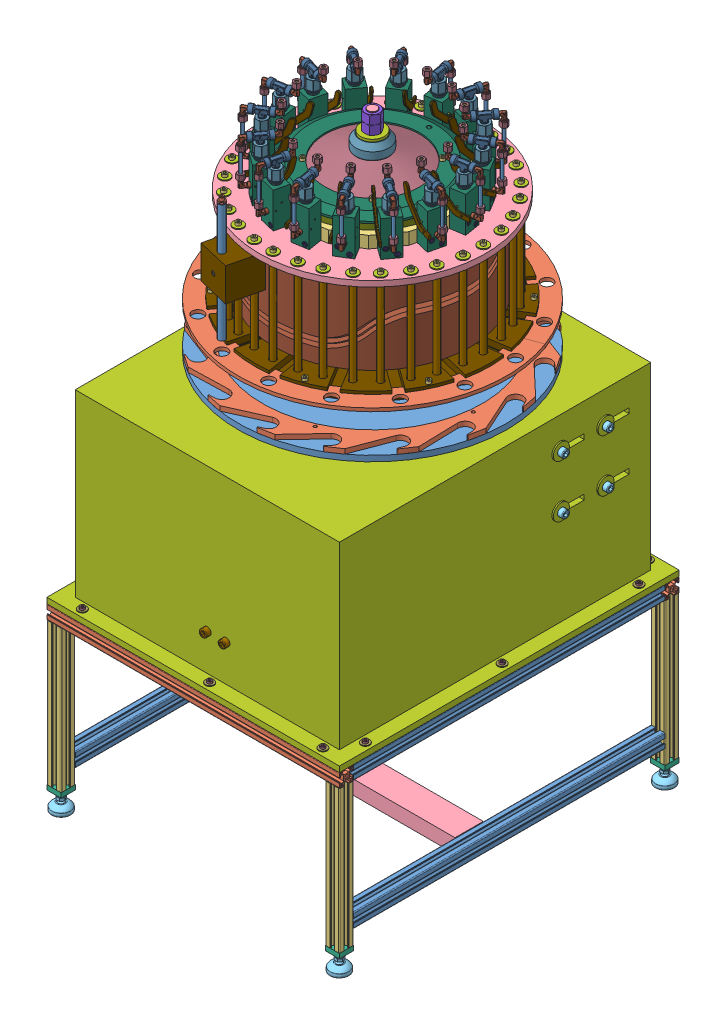
SolidWorks assembly Assieme_FINALE, configuration Default. Lengths in mm. (continued)
Components (placement in the parent): (continued)
- assieme parte rotante-2: assieme parte rotante [Default] at (-8.3038 623.9178 -528.0599) x (0 1 0) z (-0.913062 0 0.407822) size (749.63 778.63 778.63) (continued)
  - AssiemeValvola-15: AssiemeValvola [Default] at (515.3257 182.5711 371.0008) x (0 -0.965926 0.258819) z (0 0.258819 0.965926) size (90.26 138.63 38)
    - RaccordoT-1: RaccordoT [Default] at origin size (43 29.75 16.5)
    - Raccordo a L-1: Raccordo a L [Default] at (-30 0 0) x (0 -1 0) z (0 0 -1) size (28.34 25.51 14.01)
      - 1809_06_10_01-1: 1809_06_10_01 [Default] at origin size (22.49 23 10)
      - 1809_06_10_02-1: 1809_06_10_02 [Default] at origin size (6.5 8.5 8.5)
      - 1809_06_10_03-1: 1809_06_10_03 [Default] at origin size (11.02 15.01 14.01)
    - Raccordo a L-2: Raccordo a L [Default] at (30 0 0) x (0 1 0) z (0 0 -1) size (28.34 25.51 14.01)
      - 1809_06_10_01-1: 1809_06_10_01 [Default] at origin size (22.49 23 10)
      - 1809_06_10_02-1: 1809_06_10_02 [Default] at origin size (6.5 8.5 8.5)
      - 1809_06_10_03-1: 1809_06_10_03 [Default] at origin size (11.02 15.01 14.01)
    - TappoChiusura-1: TappoChiusura [Default] at (0 -32 0) x (0 -1 0) z (0 0 1) size (38.28 26.74 26.74)
    - CorpoValvola-1: CorpoValvola [Default] at (-15 -115.2824 0) size (30 75 34)
    - Raccordo a L-3: Raccordo a L [Default] at (-30 -88.2824 0) x (0 1 0) z (0 0 1) size (28.34 25.51 14.01)
      - 1809_06_10_01-1: 1809_06_10_01 [Default] at origin size (22.49 23 10)
      - 1809_06_10_02-1: 1809_06_10_02 [Default] at origin size (6.5 8.5 8.5)
      - 1809_06_10_03-1: 1809_06_10_03 [Default] at origin size (11.02 15.01 14.01)
    - Spina_3x38-1: Spina_3x38 [Default] at (0 -68.2824 -21) x (-1 0 0) z (0 0 1) size (3 3 38)
    - Spina_3x38-2: Spina_3x38 [Default] at (-10 -80.2824 -21) x (0.996193 0.087174 0) z (0 0 1) size (3 3 38)
    - M5 40mm-3: M5 40mm [ISO 4762 M5 x 40 - 40N] at (-14.6 -108.7824 9) size (45 8.5 8.5)
    - M5 40mm-2: M5 40mm [ISO 4762 M5 x 40 - 40N] at (-14.6 -96.7824 -9) size (45 8.5 8.5)
    - LevaValvola-1: LevaValvola [Default] at (-24.507 -86.571 -17) x (0.996193 0.087174 0) z (0 0 1) size (77.55 60.2 4)
    - Tubo-1: Tubo [Default] at (-30 -15.9665 0) x (1 0 0) z (0 -1 0) size (6 6 56.4)
  - AssiemeValvola-16: AssiemeValvola [Default] at (515.3257 153.2338 311.5106) x (0 -0.793353 0.608761) z (0 0.608761 0.793353) size (90.26 138.63 38)
    - RaccordoT-1: RaccordoT [Default] at origin size (43 29.75 16.5)
    - Raccordo a L-1: Raccordo a L [Default] at (-30 0 0) x (0 -1 0) z (0 0 -1) size (28.34 25.51 14.01)
      - 1809_06_10_01-1: 1809_06_10_01 [Default] at origin size (22.49 23 10)
      - 1809_06_10_02-1: 1809_06_10_02 [Default] at origin size (6.5 8.5 8.5)
      - 1809_06_10_03-1: 1809_06_10_03 [Default] at origin size (11.02 15.01 14.01)
    - Raccordo a L-2: Raccordo a L [Default] at (30 0 0) x (0 1 0) z (0 0 -1) size (28.34 25.51 14.01)
      - 1809_06_10_01-1: 1809_06_10_01 [Default] at origin size (22.49 23 10)
      - 1809_06_10_02-1: 1809_06_10_02 [Default] at origin size (6.5 8.5 8.5)
      - 1809_06_10_03-1: 1809_06_10_03 [Default] at origin size (11.02 15.01 14.01)
    - TappoChiusura-1: TappoChiusura [Default] at (0 -32 0) x (0 -1 0) z (0 0 1) size (38.28 26.74 26.74)
    - CorpoValvola-1: CorpoValvola [Default] at (-15 -115.2824 0) size (30 75 34)
    - Raccordo a L-3: Raccordo a L [Default] at (-30 -88.2824 0) x (0 1 0) z (0 0 1) size (28.34 25.51 14.01)
      - 1809_06_10_01-1: 1809_06_10_01 [Default] at origin size (22.49 23 10)
      - 1809_06_10_02-1: 1809_06_10_02 [Default] at origin size (6.5 8.5 8.5)
      - 1809_06_10_03-1: 1809_06_10_03 [Default] at origin size (11.02 15.01 14.01)
    - Spina_3x38-1: Spina_3x38 [Default] at (0 -68.2824 -21) x (-1 0 0) z (0 0 1) size (3 3 38)
    - Spina_3x38-2: Spina_3x38 [Default] at (-10 -80.2824 -21) x (0.996193 0.087174 0) z (0 0 1) size (3 3 38)
    - M5 40mm-3: M5 40mm [ISO 4762 M5 x 40 - 40N] at (-14.6 -108.7824 9) size (45 8.5 8.5)
    - M5 40mm-2: M5 40mm [ISO 4762 M5 x 40 - 40N] at (-14.6 -96.7824 -9) size (45 8.5 8.5)
    - LevaValvola-1: LevaValvola [Default] at (-24.507 -86.571 -17) x (0.996193 0.087174 0) z (0 0 1) size (77.55 60.2 4)
    - Tubo-1: Tubo [Default] at (-30 -15.9665 0) x (1 0 0) z (0 -1 0) size (6 6 56.4)
  - Disco alimentazione guarnizione fi24.4-1: Disco alimentazione guarnizione fi24.4 [Default] at (198.0433 18.3637 415) x (0 0.065403 0.997859) z (-1 0 0) size (570 285 7.35)
  - Disco alimentazione guarnizione fi24.4-2: Disco alimentazione guarnizione fi24.4 [Default] at (198.0433 18.3637 415) x (0 -0.065403 -0.997859) z (-1 0 0) size (570 285 7.35)
  - m6 12mm-1: m6 12mm [ISO 4762 M6 x 12 - 12N] at (210.0433 200.6849 574.8914) x (-1 0 0) z (0 0.793353 -0.608761) size (18 10 10)
  - m6 12mm-7: m6 12mm [ISO 4762 M6 x 12 - 12N] at (210.0433 260.3445 399.1397) x (-1 0 0) z (0 0.793353 -0.608761) size (18 10 10)
  - m6 12mm-8: m6 12mm [ISO 4762 M6 x 12 - 12N] at (210.0433 96.3128 185.3694) x (-1 0 0) z (0 0.793353 -0.608761) size (18 10 10)
  - m6 12mm-9: m6 12mm [ISO 4762 M6 x 12 - 12N] at (210.0433 -59.5854 644.6306) x (-1 0 0) z (0 -0.793353 -0.608761) size (18 10 10)
  - m6 12mm-10: m6 12mm [ISO 4762 M6 x 12 - 12N] at (210.0433 -223.6171 430.8603) x (-1 0 0) z (0 -0.793353 -0.608761) size (18 10 10)
  - m6 12mm-11: m6 12mm [ISO 4762 M6 x 12 - 12N] at (210.0433 -163.9575 255.1086) x (-1 0 0) z (0 0.793353 -0.608761) size (18 10 10)
- assieme parte fissa-1: assieme parte fissa [Default] at (-1179.2365 708.9757 -309.8267) x (0 -1 0) z (1 0 0) size (784.52 425.72 425.47)
  - AlberoPortaCamme-1: AlberoPortaCamme [Default] at (-462.1354 65.7544 784.523) size (784.52 50 50)
  - linguetta_uni_6604_a_14x9x150-1: linguetta_uni_6604_a_14x9x150 [Default] at (-282.1354 65.7544 802.023) x (1 0 0) z (0 -1 0) size (150 9 14)
  - linguetta_uni_6604_a_8x7x50-1: linguetta_uni_6604_a_8x7x50 [Default] at (-397.1354 65.7544 802.523) x (1 0 0) z (0 1 0) size (50 7 8)
  - linguetta_uni_6604_a_8x7x50-2: linguetta_uni_6604_a_8x7x50 [Default] at (-397.1354 65.7544 766.523) x (1 0 0) z (0 -1 0) size (50 7 8)
  - rondella 20d 50D 5mm-1: rondella 20d 50D 5mm [Default] at (-417.3639 65.7544 784.523) x (0 0 1) z (-1 0 0) size (50 50 5)
  - dado M20-3: dado M20 [ISO - 4034 - M20 - N] at (-441.3639 65.7544 784.523) x (0 -1 0) z (1 0 0) size (30 34.64 19)
  - dado M20-4: dado M20 [ISO - 4034 - M20 - N] at (-422.3639 65.7544 784.523) x (0 -1 0) z (1 0 0) size (30 34.64 19)
  - basic external retaining ring_am-11: basic external retaining ring_am [B27.7M - 3AM1-50] at (292.1646 65.7544 784.523) x (0 0 -1) z (1 0 0) size (54.93 58.5 1.6)
  - basic external retaining ring_am-12: basic external retaining ring_am [B27.7M - 3AM1-50] at (272.8646 65.7544 784.523) x (0 0 1) z (-1 0 0) size (54.93 58.5 1.6)
  - basic external retaining ring_am-13: basic external retaining ring_am [B27.7M - 3AM1-50] at (-120.5354 65.7544 784.523) x (0 0 -1) z (1 0 0) size (54.93 58.5 1.6)
  - basic external retaining ring_am-14: basic external retaining ring_am [B27.7M - 3AM1-50] at (-104.4354 65.7544 784.523) x (0 0 1) z (-1 0 0) size (54.93 58.5 1.6)
  - heavy duty external retaining ring_am-2: heavy duty external retaining ring_am [seger 45mm] at (-289.9354 65.7544 784.523) x (0 1 0) z (-1 0 0) size (52.13 56.09 2.8)
  - heavy duty external retaining ring_am-3: heavy duty external retaining ring_am [B27.8M - 3DM1-40] at (-342.1354 65.7544 784.523) x (0 -1 0) z (1 0 0) size (46.31 50.39 2.8)
  - camma-1: camma [Default] at (-135.1932 65.7544 784.523) x (0 1 0) z (0 0 1) size (425.72 162 425.47)
  - SKF - 6010 - 18,DE,NC,18_68-1: SKF - 6010 - 18,DE,NC,18_68 [SKF - 6010 - 18,DE,NC,18_68] at (282.5646 65.7544 784.523) size (16 80 80)
  - SKF - 6010 - 18,DE,NC,18_68-2: SKF - 6010 - 18,DE,NC,18_68 [SKF - 6010 - 18,DE,NC,18_68] at (-112.5354 65.7544 784.523) size (16 80 80)
  - assieme molla e distributore-2: assieme molla e distributore [Default] at (-388.2308 60.5069 994.523) x (0 -1 0) z (0 0 -1) size (295 75.23 295)
    - molla a tazza-1: molla a tazza [Default] at (-5.2475 5.9046 210) size (200 27.84 200)
    - flangia copertura molla-1: flangia copertura molla [Default] at (-5.2475 11.1331 210) size (70 28.5 70)
    - distributore_fisso-1: distributore_fisso [Default] at (-5.2475 -46.0954 210) x (1 0 0) z (0 1 0) size (295 295 47)
    - delring_distributore_fisso-1: delring_distributore_fisso [Default] at (-5.2475 -46.0954 210) x (0 0 1) z (0 1 0) size (295 295 12)
    - O-ring 12.5x1.8-A-ISO 3601-1-2: O-ring 12.5x1.8-A-ISO 3601-1 [O-ring 12.5x1.8-A-ISO 3601-1] at (-125.2475 -33.1954 210) x (0.868916 0 -0.49496) z (0 1 0) size (16.1 16.1 1.8)
    - M6 16mm-6: M6 16mm [ISO 4762 M6 x 16 - 16N] at (-79.4937 -15.0954 135.7538) x (0 -1 0) z (0 0 1) size (22 10 10)
    - M6 16mm-7: M6 16mm [ISO 4762 M6 x 16 - 16N] at (-79.4937 -15.0954 284.2462) x (0 -1 0) z (1 0 0) size (22 10 10)
    - M6 16mm-8: M6 16mm [ISO 4762 M6 x 16 - 16N] at (68.9987 -15.0954 284.2462) x (0 -1 0) z (0 0 -1) size (22 10 10)
    - M6 16mm-9: M6 16mm [ISO 4762 M6 x 16 - 16N] at (68.9987 -15.0954 135.7538) x (0 -1 0) z (-1 0 0) size (22 10 10)
- assieme_carrello_movimento-1: assieme_carrello_movimento [Default] at (-440.4175 901.0812 -134.2668) x (0.972647 0 0.23229) z (0 1 0) size (70 82 262.71)
  - carello movimento alternativo-1: carello movimento alternativo [Default] at (-11.6011 0.1165 35) size (70 70 70)
  - tubo_carello-1: tubo_carello [Default] at (-11.6011 -19.6699 70) x (0 -1 0) z (0 0 1) size (14 14 250)
  - raccordo dritto-1: raccordo dritto [Default] at (-11.6011 -19.6699 191.1) x (-1 0 0) z (0 1 0) size (14 16.61 13)
  - grano-1: grano [ISO 4026 - M8 x 12-N] at (-11.6011 -34.6699 70) x (0 1 0) z (0.714486 0 -0.69965) size (12 8 8)
  - Perno_folle-2: Perno_folle [Default] at (-11.6011 26.4917 70) x (0 1 0) z (0 0 1) size (32 18.94 18.94)
Mates (geometry in assembly coordinates):
- Parallelo2: parallel aligned: plane of SupportoBase_Totale-2 through (4.0127 -14.4529 -3.9361) normal (0 1 0)
- Perpendicolare1: perpendicular: plane of SupportoBase_Totale-2 through (4.0127 -14.4529 -3.9361) normal (0 1 0)
- Parallelo4: parallel aligned: plane of SupportoBase_Totale-2 through (4.0127 -14.4529 -3.9361) normal (0 0 1)
- Coincidente5: coincident anti-aligned: plane of SupportoBase_Totale-2/assieme_base-1/Supporto di Base per macchina-1 through (-154.7135 275.9611 -15.5811) normal (-1 0 0); plane of motoriduttore-1 through (-154.7135 275.9611 -1137.0941) normal (1 0 0)
- Tangente1: tangent anti-aligned: plane of SupportoBase_Totale-2/assieme_base-1/Supporto di Base per macchina-1 through (-93.2286 597.9611 -659.5811) normal (0 1 0); cylinder of motoriduttore-1 through (-154.7135 603.4611 -608.0941) axis (-1 0 0) radius 5.5
- Concentrico1: concentric anti-aligned: cylinder of motoriduttore-1 through (-267.2135 442.7547 -555.0941) axis (0 1 0) radius 15; cylinder of Assieme_Riduttore-1/AlberoRiduttore-1 through (-267.2135 379.4375 -555.0941) axis (0 -1 0) radius 12.5
- Coincidente9: coincident anti-aligned: plane of motoriduttore-1 through (-164.7135 602.1811 -1137.0941) normal (0 1 0); plane of Assieme_Riduttore-1/Rondella di fermo-2 through (-267.2135 602.1811 -555.0941) normal (0 -1 0)
- Coincidente12: coincident anti-aligned: plane of M10 50mm-1 through (-131.7135 606.5159 -520.4879) normal (-1 0 0); plane of plain washer xlarge grade c_iso-1 through (-131.7135 596.9697 -497.3823) normal (1 0 0)
- Concentrico4: concentric aligned: cylinder of M10 50mm-1 through (-89.9635 603.4611 -513.0941) axis (1 0 0) radius 5; cylinder of plain washer xlarge grade c_iso-1 through (-99.7885 603.4611 -513.0941) axis (1 0 0) radius 5.5
- Coincidente13: coincident anti-aligned: plane of M10 50mm-2 through (-131.7135 484.4611 -513.0941) normal (-1 0 0); plane of plain washer xlarge grade c_iso-2 through (-131.7135 475.4611 -513.0941) normal (1 0 0)
- Concentrico5: concentric aligned: cylinder of M10 50mm-2 through (-89.9635 492.4611 -513.0941) axis (1 0 0) radius 5; cylinder of plain washer xlarge grade c_iso-2 through (-99.7885 492.4611 -513.0941) axis (1 0 0) radius 5.5
- Coincidente14: coincident anti-aligned: plane of M10 50mm-5 through (-131.7135 595.4611 -608.0941) normal (-1 0 0); plane of plain washer xlarge grade c_iso-4 through (-131.7135 586.4611 -608.0941) normal (1 0 0)
- Concentrico6: concentric aligned: cylinder of M10 50mm-5 through (-89.9635 603.4611 -608.0941) axis (1 0 0) radius 5; cylinder of plain washer xlarge grade c_iso-4 through (-99.7885 603.4611 -608.0941) axis (1 0 0) radius 5.5
- Coincidente15: coincident anti-aligned: plane of M10 50mm-4 through (-131.7135 484.4611 -608.0941) normal (-1 0 0); plane of plain washer xlarge grade c_iso-3 through (-131.7135 475.4611 -608.0941) normal (1 0 0)
- Concentrico7: concentric aligned: cylinder of M10 50mm-4 through (-89.9635 492.4611 -608.0941) axis (1 0 0) radius 5; cylinder of plain washer xlarge grade c_iso-3 through (-99.7885 492.4611 -608.0941) axis (1 0 0) radius 5.5
- Concentrico8: concentric anti-aligned: cylinder of motoriduttore-1 through (-154.7135 603.4611 -608.0941) axis (-1 0 0) radius 5.5; cylinder of M10 50mm-5 through (-89.9635 603.4611 -608.0941) axis (1 0 0) radius 5
- Coincidente16: coincident anti-aligned: plane of SupportoBase_Totale-2/assieme_base-1/Supporto di Base per macchina-1 through (-134.7135 287.9611 -15.5811) normal (1 0 0); plane of plain washer xlarge grade c_iso-4 through (-134.7135 597.9611 -608.0941) normal (-1 0 0)
- Concentrico9: concentric anti-aligned: cylinder of motoriduttore-1 through (-154.7135 603.4611 -513.0941) axis (-1 0 0) radius 5.5; cylinder of M10 50mm-1 through (-89.9635 603.4611 -513.0941) axis (1 0 0) radius 5
- Coincidente17: coincident anti-aligned: plane of SupportoBase_Totale-2/assieme_base-1/Supporto di Base per macchina-1 through (-134.7135 287.9611 -15.5811) normal (1 0 0); plane of plain washer xlarge grade c_iso-1 through (-134.7135 601.3609 -508.0109) normal (-1 0 0)
- Coincidente18: coincident anti-aligned: plane of SupportoBase_Totale-2/assieme_base-1/Supporto di Base per macchina-1 through (-134.7135 287.9611 -15.5811) normal (1 0 0); plane of plain washer xlarge grade c_iso-3 through (-134.7135 486.9611 -608.0941) normal (-1 0 0)
- Concentrico10: concentric aligned: circle of motoriduttore-1; cylinder of M10 50mm-4 through (-89.9635 492.4611 -608.0941) axis (1 0 0) radius 5
- Coincidente19: coincident anti-aligned: plane of SupportoBase_Totale-2/assieme_base-1/Supporto di Base per macchina-1 through (-134.7135 287.9611 -15.5811) normal (1 0 0); plane of plain washer xlarge grade c_iso-2 through (-134.7135 486.9611 -513.0941) normal (-1 0 0)
- Concentrico11: concentric aligned: circle of motoriduttore-1; cylinder of M10 50mm-2 through (-89.9635 492.4611 -513.0941) axis (1 0 0) radius 5
- Concentrico12: concentric anti-aligned: cylinder of M10 50mm-4 through (-89.9635 492.4611 -608.0941) axis (1 0 0) radius 5; cylinder of hex nut style 2 gradeab_iso-7 through (-164.7135 492.4611 -608.0941) axis (-1 0 0) radius 4.25
- Coincidente20: coincident anti-aligned: plane of motoriduttore-1 through (-164.7135 275.9611 -1137.0941) normal (-1 0 0); plane of hex nut style 2 gradeab_iso-7 through (-164.7135 501.6987 -608.0941) normal (1 0 0)
- Concentrico13: concentric anti-aligned: cylinder of M10 50mm-5 through (-89.9635 603.4611 -608.0941) axis (1 0 0) radius 5; cylinder of hex nut style 2 gradeab_iso-5 through (-164.7135 603.4611 -608.0941) axis (-1 0 0) radius 4.25
- Coincidente21: coincident aligned: plane of motoriduttore-1 through (-164.7135 275.9611 -1137.0941) normal (-1 0 0); circle of hex nut style 2 gradeab_iso-1
- Concentrico14: concentric anti-aligned: cylinder of M10 50mm-1 through (-89.9635 603.4611 -513.0941) axis (1 0 0) radius 5; cylinder of hex nut style 2 gradeab_iso-8 through (-164.7135 603.4611 -513.0941) axis (-1 0 0) radius 4.25
- Coincidente22: coincident anti-aligned: plane of motoriduttore-1 through (-164.7135 275.9611 -1137.0941) normal (-1 0 0); plane of hex nut style 2 gradeab_iso-8 through (-164.7135 612.6987 -513.0941) normal (1 0 0)
- Concentrico15: concentric anti-aligned: cylinder of M10 50mm-2 through (-89.9635 492.4611 -513.0941) axis (1 0 0) radius 5; cylinder of hex nut style 2 gradeab_iso-6 through (-164.7135 492.4611 -513.0941) axis (-1 0 0) radius 4.25
- Coincidente23: coincident anti-aligned: plane of motoriduttore-1 through (-164.7135 275.9611 -1137.0941) normal (-1 0 0); plane of hex nut style 2 gradeab_iso-6 through (-164.7135 501.6987 -513.0941) normal (1 0 0)
- Concentrico164: concentric anti-aligned: cylinder of SupportoBase_Totale-2/assieme_base-1/Traversa di blocco albero-1 through (-394.7135 362.1119 -360.5811) axis (0 1 0) radius 5.25; cylinder of assieme parte fissa-1/AlberoPortaCamme-1 through (-394.7135 386.9611 -360.5811) axis (0 -1 0) radius 4.5
- Coincidente26: coincident anti-aligned: plane of SupportoBase_Totale-2/assieme_base-1/Traversa di blocco albero-1 through (-427.2135 386.9611 -53.5811) normal (0 1 0); plane of assieme parte fissa-1/AlberoPortaCamme-1 through (-394.7135 386.9611 -400.5811) normal (0 -1 0)
- Concentrico1651: concentric aligned: cylinder of SupportoBase_Totale-2/assieme_base-1/Traversa di blocco albero-1 through (-394.7135 362.1119 -360.5811) axis (0 1 0) radius 5.25; cylinder of rondella M8-1 through (-394.7135 374.9611 -360.5811) axis (0 1 0) radius 4.65
- Coincidente271: coincident anti-aligned: plane of SupportoBase_Totale-2/assieme_base-1/Traversa di blocco albero-1 through (-427.2135 376.9611 -53.5811) normal (0 -1 0); plane of rondella M8-1 through (-394.7135 376.9611 -360.5811) normal (0 1 0)
- Concentrico1661: concentric aligned: cylinder of SupportoBase_Totale-2/assieme_base-1/Traversa di blocco albero-1 through (-394.7135 362.1119 -390.5811) axis (0 1 0) radius 5.25; cylinder of rondella M8-2 through (-394.7135 374.9611 -390.5811) axis (0 1 0) radius 4.65
- Coincidente281: coincident anti-aligned: plane of SupportoBase_Totale-2/assieme_base-1/Traversa di blocco albero-1 through (-427.2135 376.9611 -53.5811) normal (0 -1 0); plane of rondella M8-2 through (-394.7135 376.9611 -390.5811) normal (0 1 0)
- Coincidente29: coincident aligned: plane of rondella M8-1 through (-394.7135 376.9611 -360.5811) normal (-1 0 0); plane of rondella M8-2 through (-394.7135 376.9611 -390.5811) normal (-1 0 0)
- Concentrico16621: concentric anti-aligned: cylinder of SupportoBase_Totale-2/assieme_base-1/Traversa di blocco albero-1 through (-394.7135 362.1119 -390.5811) axis (0 1 0) radius 5.25; cylinder of M8 25 mm-1 through (-394.7135 337.2111 -390.5811) axis (0 -1 0) radius 6.5
- Coincidente2821: coincident anti-aligned: plane of SupportoBase_Totale-2/assieme_base-1/Traversa di blocco albero-1 through (-427.2135 376.9611 -53.5811) normal (0 -1 0); plane of M8 25 mm-1 through (-400.3427 376.9611 -387.3311) normal (0 1 0)
- Concentrico16631: concentric anti-aligned: cylinder of rondella M8-1 through (-394.7135 374.9611 -360.5811) axis (0 1 0) radius 4.65; cylinder of M8 25 mm-2 through (-394.7135 335.2111 -360.5811) axis (0 -1 0) radius 6.5
- Coincidente284: coincident anti-aligned: plane of rondella M8-1 through (-394.7135 374.9611 -360.5811) normal (0 -1 0); plane of M8 25 mm-2 through (-389.0844 374.9611 -363.8311) normal (0 1 0)
- Coincidente285: coincident aligned: plane of M8 25 mm-1 through (-391.666 372.9611 -388.8216) normal (-1 0 0); plane of M8 25 mm-2 through (-391.666 370.9611 -362.3406) normal (-1 0 0)
- Concentrico16632: concentric aligned: cylinder of assieme parte rotante-1/asta scorrimento carello-15 through (-613.1413 1023.9611 -329.7302) axis (0 -1 0) radius 6; cylinder of assieme_carrello_movimento-1/carello movimento alternativo-1 through (-423.911 1006.0812 -154.3109) axis (0 -1 0) radius 7
- Concentrico16635: concentric anti-aligned: cylinder of assieme parte rotante-1/asta scorrimento carello-30 through (-617.9018 798.9611 -375.4832) axis (0 1 0) radius 6; cylinder of assieme_carrello_movimento-1/carello movimento alternativo-1 through (-468.6528 1006.0812 -164.9962) axis (0 -1 0) radius 7
- Concentrico16648: concentric aligned: cylinder of assieme parte fissa-1/AlberoPortaCamme-1 through (-394.7135 1275.1556 -375.5811) axis (0 1 0) radius 25; cylinder of assieme parte rotante-2/albero rotazione piatti-1 through (-394.7135 684.3308 -375.5811) axis (0 1 0) radius 35
- Coincidente2822: coincident anti-aligned: plane of SupportoBase_Totale-2/assieme_base-1/canotto di supporto-1 through (-394.7135 673.9611 -375.5811) normal (0 1 0); plane of assieme parte rotante-2/SKF - 6020 - 20,DE,NC,20_68-2 through (-396.2853 673.9611 -318.1026) normal (0 -1 0)
- Concentrico16650: concentric aligned: cylinder of SupportoBase_Totale-2/assieme_base-1/canotto di supporto-1 through (-394.7135 587.1745 -375.5811) axis (0 1 0) radius 67.5; cylinder of assieme parte fissa-1/AlberoPortaCamme-1 through (-394.7135 1275.1556 -375.5811) axis (0 1 0) radius 25
- Concentrico16651: concentric anti-aligned: cylinder of assieme parte rotante-2/asta scorrimento carello-23 through (-468.6528 798.9611 -164.9962) axis (0 1 0) radius 6; cylinder of assieme_carrello_movimento-1/carello movimento alternativo-1 through (-468.6528 1006.0812 -164.9962) axis (0 -1 0) radius 7
- Concentrico16652: concentric aligned: cylinder of assieme parte rotante-2/asta scorrimento carello-8 through (-423.911 1023.9611 -154.3109) axis (0 -1 0) radius 6; cylinder of assieme_carrello_movimento-1/carello movimento alternativo-1 through (-423.911 1006.0812 -154.3109) axis (0 -1 0) radius 7
- Tangente8: tangent: face of assieme parte fissa-1/camma-1; cylinder of ? through (-185.8875 941.1413 -276.1155) axis (0.902819 0 0.430021) radius 9.47
